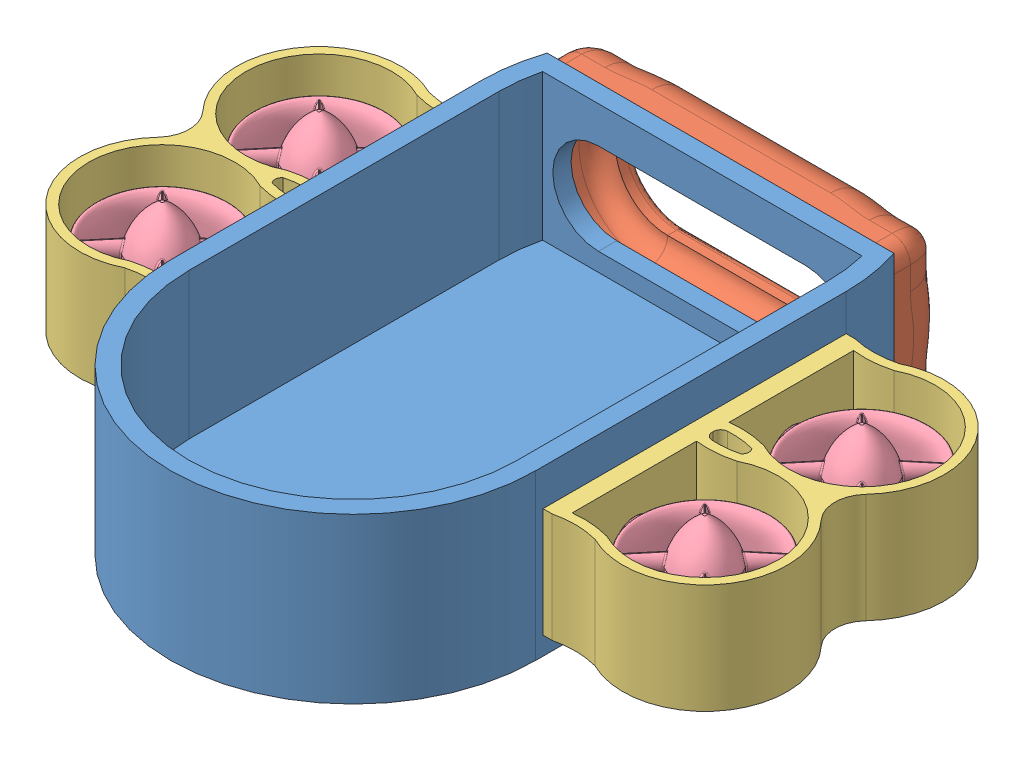
SolidWorks assembly Assem1, configuration Default. Lengths in mm.
Overall size (492.12 136.15 420.66).
10 component instances, 4 part files, 10 mates.
Components (placement in the parent):
- Pink-2: Pink [Default] at (-144.9815 380.0297 -29.3812) size (254 114.3 382.56)
- PinkTestPlate-1: PinkTestPlate [Default] at (-144.9815 437.1797 -176.987) x (1 0 0) z (0 1 0) size (241.3 38.1 114.3)
- CR-A-0004b-VerticalMotorAssem-1: CR-A-0004b-VerticalMotorAssem [Default] at (-399.546 651.6874 -200.5213) x (1 0 0) z (0 -1 0) size (119.06 223.52 112.68)
  - CR-P-0005b-Frame-MotorMount Vertical-1: CR-P-0005b-Frame-MotorMount Vertical [Default] at (65.652 113.9901 182.7577) size (119.06 223.52 76.2)
  - CR-P-0003-T200-THRUSTER-R1-1: CR-P-0003-T200-THRUSTER-R1 [Default] at (65.8645 223.2101 226.1095) x (0 -1 0) z (0 0 1) size (96.71 97.53 112.68)
  - CR-P-0003-T200-THRUSTER-R1-2: CR-P-0003-T200-THRUSTER-R1 [Default] at (65.8645 113.9901 226.1095) x (0 -1 0) z (0 0 1) size (96.71 97.53 112.68)
- CR-A-0004b-VerticalMotorAssem-2: CR-A-0004b-VerticalMotorAssem [Default] at (109.583 651.6874 136.6788) x (-1 0 0) z (0 -1 0) size (119.06 223.52 112.68)
  - CR-P-0005b-Frame-MotorMount Vertical-1: CR-P-0005b-Frame-MotorMount Vertical [Default] at (65.652 113.9901 182.7577) size (119.06 223.52 76.2)
  - CR-P-0003-T200-THRUSTER-R1-1: CR-P-0003-T200-THRUSTER-R1 [Default] at (65.8645 223.2101 226.1095) x (0 -1 0) z (0 0 1) size (96.71 97.53 112.68)
  - CR-P-0003-T200-THRUSTER-R1-2: CR-P-0003-T200-THRUSTER-R1 [Default] at (65.8645 113.9901 226.1095) x (0 -1 0) z (0 0 1) size (96.71 97.53 112.68)
Mates (geometry in assembly coordinates):
- Coincident4: coincident aligned: plane of Pink-2 through (-144.9815 494.3297 -29.3812) normal (0 1 0); plane of PinkTestPlate-1 through (-265.6315 494.3297 -215.087) normal (0 1 0)
- Coincident5: coincident anti-aligned: plane of Pink-2 through (-144.9815 494.3297 -176.987) normal (0 0 -1); plane of PinkTestPlate-1 through (-144.9815 437.1797 -176.987) normal (0 0 1)
- Coincident6: coincident anti-aligned: line of Pink-2 through (-265.6315 494.3297 -176.987) axis (0 -1 0); line of PinkTestPlate-1 through (-265.6315 392.7297 -176.987) axis (0 1 0)
- Coincident7: coincident anti-aligned: plane of Pink-2 through (-271.9815 494.3297 -29.3812) normal (-1 0 0); plane of CR-A-0004b-VerticalMotorAssem-1/CR-P-0005b-Frame-MotorMount Vertical-1 through (-271.9815 468.9297 -86.5312) normal (1 0 0)
- Coincident8: coincident anti-aligned: plane of Pink-2 through (-271.9815 494.3297 -29.3812) normal (-1 0 0); plane of CR-A-0004b-VerticalMotorAssem-1/CR-P-0005b-Frame-MotorMount Vertical-1 through (-271.9815 468.9297 -86.5312) normal (1 0 0)
- Coincident10: coincident: line of Pink-2 through (-271.9815 494.3297 -137.3312) axis (0 -1 0); plane of CR-A-0004b-VerticalMotorAssem-1/CR-P-0005b-Frame-MotorMount Vertical-1 through (-271.9815 468.9297 -137.3312) normal (0 0 -1)
- Distance1: distance = 12.7 mm aligned: plane of CR-A-0004b-VerticalMotorAssem-1/CR-P-0005b-Frame-MotorMount Vertical-1 through (-333.894 392.7297 -86.5312) normal (0 -1 0); plane of Pink-2 through (-144.9815 380.0297 -29.3812) normal (0 -1 0)
- Coincident12: coincident anti-aligned: plane of Pink-2 through (-17.9815 494.3297 -29.3812) normal (1 0 0); plane of CR-A-0004b-VerticalMotorAssem-2/CR-P-0005b-Frame-MotorMount Vertical-1 through (-17.9815 468.9297 22.6888) normal (-1 0 0)
- Distance2: distance = 12.7 mm aligned: plane of CR-A-0004b-VerticalMotorAssem-2/CR-P-0005b-Frame-MotorMount Vertical-1 through (43.931 392.7297 22.6888) normal (0 -1 0); plane of Pink-2 through (-144.9815 380.0297 -29.3812) normal (0 -1 0)
- Coincident14: coincident: line of Pink-2 through (-17.9815 494.3297 -137.3312) axis (0 -1 0); plane of CR-A-0004b-VerticalMotorAssem-2/CR-P-0005b-Frame-MotorMount Vertical-1 through (-17.9815 468.9297 -137.3312) normal (0 0 -1)
